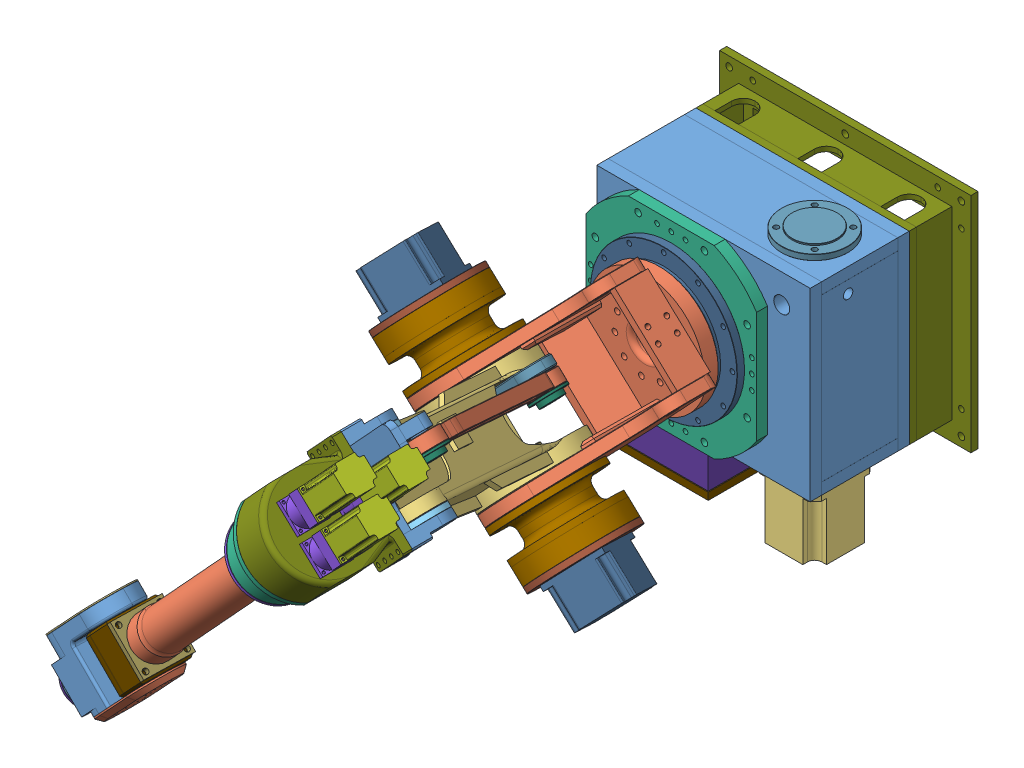
SolidWorks assembly CHX-3装配图, configuration 默认. Lengths in mm.
Overall size (845.77 871.93 1351.14).
99 component instances, 76 part files, 255 mates.
Components (placement in the parent):
- CHX-3底盘旋转涡轮箱-1: CHX-3底盘旋转涡轮箱 [默认] at (-163.7739 242.4792 201.5814) size (450 390 209)
- CHX-3驱动臂座-1: CHX-3驱动臂座 [默认] at (16.2261 47.4792 428.5814) x (-0.730588 0.682819 0) z (0 0 1) size (250 411.05 303.07)
- CHX-3大手臂2-1: CHX-3大手臂2 [默认] at (-120.8336 -194.3627 713.0096) x (0.515271 0.551318 -0.656159) z (-0.730588 0.682819 0) size (210 817.13 178)
- CHX-3小手臂关节轴承-1: CHX-3小手臂关节轴承 [默认] at (145.4781 253.1428 1173.5815) x (0.49992 0.534894 -0.681152) z (-0.730588 0.682819 0) size (72 72 19)
- CHX-3小手臂关节轴承-2: CHX-3小手臂关节轴承 [默认] at (212.6936 190.3221 1173.5815) x (-0.682714 -0.730476 0.017502) z (0.730588 -0.682819 0) size (72 72 19)
- CHX-3小手臂关节轴芯-1: CHX-3小手臂关节轴芯 [默认] at (212.6936 190.3221 1173.5815) x (0.677165 0.724539 0.128414) z (0.730588 -0.682819 0) size (95 95 31)
- CHX-3小手臂关节轴芯-2: CHX-3小手臂关节轴芯 [默认] at (145.4781 253.1428 1173.5815) x (-0.40576 -0.434146 -0.804286) z (-0.730588 0.682819 0) size (95 95 31)
- CHX-3小手臂旋转轴主动齿轮-1: CHX-3小手臂旋转轴主动齿轮 [默认] at (221.5211 267.135 1289.3662) x (0.727771 -0.633712 -0.262218) z (0.677165 0.724539 0.128414) size (28.4 28.27 47)
- CHX-3旋转臂电机-1: CHX-3旋转臂电机 [默认] at (320.3993 416.8662 1282.0229) x (-0.087684 -0.093818 0.991721) z (-0.677165 -0.724539 -0.128414) size (60 60 154.5)
- CHX-3腕部行星减速机-3: CHX-3腕部行星减速机 [默认] at (182.5962 269.4225 1255.8906) x (0.730588 -0.682819 0) z (0.677165 0.724539 0.128414) size (60 60 114)
- CHX-3TVM-611摆线减速机-1: CHX-3TVM-611摆线减速机 [默认] at (-15.3461 -170.831 657.6504) x (0.682819 0.730588 0) z (-0.730588 0.682819 0) size (210 210 176)
- CHX-3TVM-611摆线减速机-2: CHX-3TVM-611摆线减速机 [默认] at (-199.4543 1.2393 657.6504) x (-0.341409 -0.365294 -0.866025) z (0.730588 -0.682819 0) size (210 210 176)
- CHX-3连杆伺服电机-2: CHX-3连杆伺服电机 [默认] at (3.9396 -301.0414 635.6889) x (0.341409 0.365294 0.866025) z (0.730588 -0.682819 0) size (120 120 126.5)
- CHX-3连杆伺服电机-3: CHX-3连杆伺服电机 [默认] at (-259.7091 87.6144 575.6889) x (0.341409 0.365294 0.866025) z (-0.730588 0.682819 0) size (120 120 126.5)
- CHX-3大手臂摆线减速机安装法兰-1: CHX-3大手臂摆线减速机安装法兰 [默认] at (-274.7048 71.5696 657.6504) x (0.341409 0.365294 0.866025) z (0.730588 -0.682819 0) size (204 204 16)
- CHX-3大手臂摆线减速机安装法兰-2: CHX-3大手臂摆线减速机安装法兰 [默认] at (59.9045 -241.1613 657.6504) x (0.341409 0.365294 0.866025) z (-0.730588 0.682819 0) size (204 204 16)
- CHX-3大手臂摆线减速机手臂安装法兰-1: CHX-3大手臂摆线减速机手臂安装法兰 [默认] at (-35.072 -152.3949 657.6504) x (0.669196 0.716013 0.198752) z (-0.730588 0.682819 0) size (135 135 55)
- CHX-3连杆轴承套-1: CHX-3连杆轴承套 [默认] at (-139.546 -54.7518 657.6504) x (0.341409 0.365294 0.866025) z (-0.730588 0.682819 0) size (67 67 55)
- CHX-3连杆轴传动轴-1: CHX-3连杆轴传动轴 [默认] at (-149.0437 -45.8752 657.6504) x (0.678123 0.725564 0.117075) z (0.730588 -0.682819 0) size (235 70 59)
- CHX-3连杆轴承盖-1: CHX-3连杆轴承盖 [默认] at (278.7548 340.0903 1206.6991) x (0.418074 0.447322 0.790644) z (0.730588 -0.682819 0) size (70 70 15)
- CHX-3连杆轴承盖-2: CHX-3连杆轴承盖 [默认] at (-1.3546 40.3847 676.9678) x (0.258501 0.276586 -0.925569) z (0.730588 -0.682819 0) size (70 70 15)
- CHX-3旋转臂电机-2: CHX-3旋转臂电机 [默认] at (286.259 423.5253 1424.4823) x (0.730588 -0.682819 0) z (-0.677165 -0.724539 -0.128414) size (60 60 154.5)
- CHX-3旋转臂电机-3: CHX-3旋转臂电机 [默认] at (343.1408 380.3198 1368.3026) x (-0.087684 -0.093818 0.991721) z (-0.677165 -0.724539 -0.128414) size (60 60 154.5)
- CHX-3腕部行星减速机-4: CHX-3腕部行星减速机 [默认] at (200.0766 227.247 1401.6735) x (0.087684 0.093818 -0.991721) z (0.677165 0.724539 0.128414) size (60 60 114)
- CHX-3腕部行星减速机-5: CHX-3腕部行星减速机 [默认] at (192.2911 235.1125 1398.35) x (-0.730588 0.682819 0) z (0.677165 0.724539 0.128414) size (60 60 114)
- CHX-3腕部电机齿轮箱-1: CHX-3腕部电机齿轮箱 [默认] at (196.3592 240.2128 1348.1206) x (0.730588 -0.682819 0) z (-0.677165 -0.724539 -0.128414) size (210 204.85 98.31)
- CHX-3手腕直齿1-1: CHX-3手腕直齿1 [默认] at (163.8553 205.4349 1341.9567) x (0.440791 -0.259684 -0.859225) z (-0.677165 -0.724539 -0.128414) size (67.8 67.8 20)
- CHX-3手腕直齿3-1: CHX-3手腕直齿3 [默认] at (179.4301 222.0993 1344.9102) x (0.474267 -0.296326 -0.829013) z (-0.677165 -0.724539 -0.128414) size (43.65 43.65 20)
- CHX-3手腕直齿4-1: CHX-3手腕直齿4 [默认] at (192.1209 174.7991 1365.758) x (-0.034964 0.206002 -0.977927) z (-0.677165 -0.724539 -0.128414) size (35.54 35.54 20)
- CHX-3手腕直齿4-2: CHX-3手腕直齿4 [默认] at (153.8046 194.6811 1276.5248) x (0.713515 -0.603899 -0.355249) z (-0.677165 -0.724539 -0.128414) size (35.54 35.54 20)
- CHX-3手腕直齿4-3: CHX-3手腕直齿4 [默认] at (156.0749 240.2981 1365.388) x (-0.708628 0.59511 0.379066) z (-0.677165 -0.724539 -0.128414) size (35.54 35.54 20)
- CHX-3腕部中心轴1-2: CHX-3腕部中心轴1 [默认] at (159.7923 201.0877 1341.1862) x (-0.103765 -0.078746 0.99148) z (-0.677165 -0.724539 -0.128414) size (98 98 563)
- CHX-3腕部中心轴2-1: CHX-3腕部中心轴2 [默认] at (191.6191 235.141 1347.2217) x (0.72823 -0.634867 -0.258119) z (-0.677165 -0.724539 -0.128414) size (20 20 703)
- CHX-3腕部中心轴3-1: CHX-3腕部中心轴3 [默认] at (170.6269 212.6803 1343.2408) x (-0.440791 0.259684 0.859225) z (-0.677165 -0.724539 -0.128414) size (50 50 657.3)
- CHX-3轴承1-1: CHX-3轴承1 [默认] at (129.3199 168.4834 1335.4076) x (0.59922 -0.644269 0.475239) z (-0.677165 -0.724539 -0.128414) size (125 125 18)
- CHX-3轴承1-2: CHX-3轴承1 [默认] at (83.2726 119.2148 1326.6754) x (0.714057 -0.604903 -0.352441) z (-0.677165 -0.724539 -0.128414) size (125 125 18)
- CHX-3小手臂旋转法兰-3: CHX-3小手臂旋转法兰 [默认] at (132.0285 171.3816 1335.9212) x (0.087684 0.093818 -0.991721) z (-0.677165 -0.724539 -0.128414) size (200 180 97)
- CHX-3手腕直齿2-1: CHX-3手腕直齿2 [默认] at (148.2805 188.7705 1339.0032) x (0.441739 -0.539852 0.716538) z (0.677165 0.724539 0.128414) size (97.98 97.94 20)
- CHX-3小手臂旋转轴承法兰-1: CHX-3小手臂旋转轴承法兰 [默认] at (69.7293 104.724 1324.1071) x (0.578605 -0.416486 -0.701252) z (-0.677165 -0.724539 -0.128414) size (155 155 33)
- CHX-3小手臂旋转后法兰-1: CHX-3小手臂旋转后法兰 [默认] at (134.7372 174.2798 1336.4349) x (0.441739 -0.539852 0.716538) z (0.677165 0.724539 0.128414) size (95 95 32)
- CHX-3手腕电机齿轮连接轴-1: CHX-3手腕电机齿轮连接轴 [默认] at (221.239 205.9543 1371.2798) x (0.022963 -0.195239 0.980487) z (-0.677165 -0.724539 -0.128414) size (25 25 53)
- CHX-3手腕电机齿轮连接轴2-1: CHX-3手腕电机齿轮连接轴2 [默认] at (198.4975 242.5007 1285.0001) x (-0.590396 0.639148 -0.492872) z (-0.677165 -0.724539 -0.128414) size (29 29 76)
- CHK-3前爪固定座-2: CHK-3前爪固定座 [默认] at (-245.1525 -232.1867 1264.3944) x (-0.728478 0.68472 -0.021858) z (-0.677165 -0.724539 -0.128414) size (100 100 15.5)
- CHX-3手腕大齿2-1: CHX-3手腕大齿2 [默认] at (-293.2061 -283.602 1255.2818) x (0.440791 -0.259684 -0.859225) z (-0.677165 -0.724539 -0.128414) size (82.68 82.68 53.06)
- CHX-3手腕61908轴承-2: CHX-3手腕61908轴承 [默认] at (-237.0265 -223.4922 1265.9354) x (0.683643 -0.554933 -0.474006) z (-0.677165 -0.724539 -0.128414) size (68 68 12)
- CHX-3手腕61908轴承-3: CHX-3手腕61908轴承 [默认] at (125.2569 164.1362 1334.6371) x (0.658688 -0.519082 -0.544688) z (-0.677165 -0.724539 -0.128414) size (68 68 12)
- CHX-3手腕61908轴承-4: CHX-3手腕61908轴承 [默认] at (-228.9006 -214.7978 1267.4764) x (0.668303 -0.532552 -0.519384) z (-0.677165 -0.724539 -0.128414) size (68 68 12)
- CHX-3手腕61908轴承-5: CHX-3手腕61908轴承 [默认] at (133.3829 172.8307 1336.1781) x (-0.154974 0.311031 -0.937679) z (-0.677165 -0.724539 -0.128414) size (68 68 12)
- CHX-3手腕6002轴承-1: CHX-3手腕6002轴承 [默认] at (164.5325 206.1595 1342.0851) x (0.732546 -0.680269 -0.024713) z (-0.677165 -0.724539 -0.128414) size (32 32 9)
- CHX-3手腕6002轴承-2: CHX-3手腕6002轴承 [默认] at (170.6269 212.6803 1343.2408) x (0.712808 -0.689224 0.129899) z (-0.677165 -0.724539 -0.128414) size (32 32 9)
- CHX-3手腕61902轴承-1: CHX-3手腕61902轴承 [默认] at (-264.9935 -253.4157 1260.6319) x (0.600589 -0.443395 -0.665352) z (-0.677165 -0.724539 -0.128414) size (28 28 7)
- CHX-3手腕61902轴承-2: CHX-3手腕61902轴承 [默认] at (-269.7336 -258.4875 1259.733) x (-0.283367 0.41783 -0.863204) z (-0.677165 -0.724539 -0.128414) size (28 28 7)
- CHX-3手腕小齿-1: CHX-3手腕小齿 [默认] at (-293.2313 -283.629 1255.277) x (-0.601822 0.645756 -0.469905) z (-0.677165 -0.724539 -0.128414) size (42.49 42.49 27.7)
- CHK-3前爪法兰-1: CHK-3前爪法兰 [默认] at (-214.4458 -289.7986 1318.5051) x (-0.677165 -0.724539 -0.128414) z (-0.728478 0.68472 -0.021858) size (112 110 108)
- CHX-3手腕前端旋转法兰-1: CHX-3手腕前端旋转法兰 [默认] at (-315.9608 -183.9595 1200.5471) x (0.728478 -0.68472 0.021858) z (-0.042031 -0.012825 0.999034) size (141 200 110)
- CHK-3前爪法兰侧盖-1: CHK-3前爪法兰侧盖 [默认] at (-305.2348 -395.7723 1253.3323) x (0.683779 0.728693 0.038123) z (-0.728478 0.68472 -0.021858) size (200 110 13)
- CHK-3前爪法兰侧钣金盖-1: CHK-3前爪法兰侧钣金盖 [默认] at (-418.8774 -288.9559 1249.9225) x (0.683779 0.728693 0.038123) z (0.728478 -0.68472 0.021858) size (200 110 2)
- CHX-3小手腕旋转齿轮-2: CHX-3小手腕旋转齿轮 [默认] at (-347.5029 -232.6173 1253.6486) x (0.638355 0.690038 0.341101) z (0.728478 -0.68472 0.021858) size (93.98 93.93 15)
- CHX-3手腕大齿-2-1: CHX-3手腕大齿-2 [默认] at (-293.1855 -283.672 1255.2784) x (0.683779 0.728693 0.038123) z (0.728478 -0.68472 0.021858) size (82.68 82.68 55.06)
- CHX-3手腕轴1-1: CHX-3手腕轴1 [默认] at (-302.4829 -274.933 1254.9994) x (0.638355 0.690038 0.341101) z (-0.728478 0.68472 -0.021858) size (20 20 69.3)
- CHX-3手腕前爪连接轴-1: CHX-3手腕前爪连接轴 [默认] at (-261.9067 -313.072 1256.2169) x (0.683779 0.728693 0.038123) z (0.728478 -0.68472 0.021858) size (62 62 19)
- CHX-3手腕前端锥齿2-1: CHX-3手腕前端锥齿2 [默认] at (-354.7713 -349.2113 1251.846) x (-0.57505 0.570294 -0.586585) z (0.683779 0.728693 0.038123) size (52.79 52.7 37)
- CHX-3小手腕旋转齿轮-2-1: CHX-3小手腕旋转齿轮-2 [默认] at (-409.0429 -298.1997 1250.2175) x (0.655459 0.687358 -0.312909) z (-0.728478 0.68472 -0.021858) size (93.98 93.93 15)
- CHX-3小手腕锥齿轮旋转中心轴-1: CHX-3小手腕锥齿轮旋转中心轴 [默认] at (-414.5065 -293.0643 1250.0536) x (0.655459 0.687358 -0.312909) z (0.728478 -0.68472 0.021858) size (39 39 145)
- CHX-3手腕6007轴承-1: CHX-3手腕6007轴承 [默认] at (-395.5661 -310.867 1250.6219) x (-0.600116 -0.653205 -0.461719) z (-0.728478 0.68472 -0.021858) size (62 62 9)
- CHX-3手腕6204轴承-1: CHX-3手腕6204轴承 [默认] at (-328.5461 -373.8613 1252.6329) x (0.231702 0.276284 0.932728) z (0.728478 -0.68472 0.021858) size (47 47 14)
- CHX-3手腕16011轴承-1: CHX-3手腕16011轴承 [默认] at (-261.9067 -313.072 1256.2169) x (0.164462 0.205767 0.964682) z (0.728478 -0.68472 0.021858) size (90 90 11)
- CHX-3手腕16011轴承-2: CHX-3手腕16011轴承 [默认] at (-332.5691 -246.6541 1254.0967) x (0.272826 0.319233 0.907555) z (0.728478 -0.68472 0.021858) size (90 90 11)
- CHX-3小手腕前端法兰-1: CHX-3小手腕前端法兰 [默认] at (-399.2169 -396.5764 1249.368) x (0.042031 0.012825 -0.999034) z (0.683779 0.728693 0.038123) size (90 90 33)
- CHX-3腕部前端中心轴-1: CHX-3腕部前端中心轴 [默认] at (-366.3956 -361.5991 1251.1979) x (0.57505 -0.570294 0.586585) z (-0.683779 -0.728693 -0.038123) size (60 60 71)
- CHX-3手腕小齿-2: CHX-3手腕小齿 [默认] at (-293.2313 -283.629 1255.277) x (0.638355 0.690038 0.341101) z (0.728478 -0.68472 0.021858) size (42.49 42.49 27.7)
- CHX-3小手臂骨架油封-1: CHX-3小手臂骨架油封 [默认] at (56.8632 90.9578 1321.6672) x (-0.503239 0.583332 -0.637554) z (-0.677165 -0.724539 -0.128414) size (105 105 12)
- CHX-3手腕前端轴承顶套-1: CHX-3手腕前端轴承顶套 [默认] at (-408.7899 -406.7781 1248.8343) x (-0.728478 0.68472 -0.021858) z (0.683779 0.728693 0.038123) size (90 90 16)
- CHX-3手腕前端锥齿1-1: CHX-3手腕前端锥齿1 [默认] at (-354.7713 -349.2113 1251.846) x (-0.655459 -0.687358 0.312909) z (0.728478 -0.68472 0.021858) size (52.79 52.7 37)
- CHX-3腕部中心轴骨架油封-2: CHX-3腕部中心轴骨架油封 [默认] at (-401.9521 -399.4912 1249.2155) x (0.553474 -0.551989 0.623678) z (-0.683779 -0.728693 -0.038123) size (55 55 10)
- CHX-3手腕61907轴承-1: CHX-3手腕61907轴承 [默认] at (-386.9089 -383.4599 1250.0542) x (0.266768 -0.298271 0.916444) z (0.683779 0.728693 0.038123) size (55 55 10)
- CHX-3手腕61907轴承-2: CHX-3手腕61907轴承 [默认] at (-397.8494 -395.119 1249.4442) x (0.266768 -0.298271 0.916444) z (0.683779 0.728693 0.038123) size (55 55 10)
- CHX-3底盘旋转电机SGMGH-13A-B键8X7-1: CHX-3底盘旋转电机SGMGH-13A-B键8X7 [默认] at (256.2261 -170.5208 371.0814) x (0 0 -1) z (0 -1 0) size (130 130 197)
- CHX-3底盘旋转涡轮-1: CHX-3底盘旋转涡轮 [默认] at (16.2261 47.4792 306.0814) x (-0.730588 0.682819 0) z (0 0 -1) size (320.22 320.22 100)
- CHX-3底盘旋转涡杆-1: CHX-3底盘旋转涡杆 [默认] at (191.2261 45.9792 306.0814) x (0.906678 0 -0.421823) z (0 -1 0) size (64 64 391.5)
- CHX-3底盘法兰盖-1: CHX-3底盘法兰盖 [默认] at (36.2261 42.4792 410.5814) size (360 390 23)
- CHX-3底盘旋转涡轮轴-1: CHX-3底盘旋转涡轮轴 [默认] at (16.2261 47.4792 368.0814) x (-0.730588 0.682819 0) z (0 0 -1) size (175 175 332)
- CHX-3底盘旋转涡轮轴下法兰-1: CHX-3底盘旋转涡轮轴下法兰 [默认] at (16.2261 47.4792 227.5814) x (-0.809017 -0.587785 0) z (0 0 -1) size (205 205 79)
- CHX-3底盘旋转51315轴承-2: CHX-3底盘旋转51315轴承 [默认] at (16.2261 47.4792 239.0814) x (0.990498 0.137527 0) z (0 0 1) size (135 135 44)
- CHX-3底盘旋转涡轮轴上法兰盖-1: CHX-3底盘旋转涡轮轴上法兰盖 [默认] at (16.2261 47.4792 449.5814) x (0 -1 0) z (0 0 -1) size (310 310 66)
- CHX-3底盘旋转涡轮轴上法兰16032轴承-2: CHX-3底盘旋转涡轮轴上法兰16032轴承 [默认] at (16.2261 47.4792 396.5814) size (240 240 38)
- CHX-3底盘旋转涡轮轴下法兰6215轴承-1: CHX-3底盘旋转涡轮轴下法兰6215轴承 [默认] at (16.2261 47.4792 153.5814) x (0.976634 0.214912 0) z (0 0 1) size (115 115 20)
- CHX-3底盘旋转涡轮轴下法兰6215轴承-2: CHX-3底盘旋转涡轮轴下法兰6215轴承 [默认] at (16.2261 47.4792 173.5814) size (115 115 20)
- CHX-3底盘旋转涡轮轴上法兰油封-1: CHX-3底盘旋转涡轮轴上法兰油封 [默认] at (16.2261 47.4792 441.5814) size (190 190 14)
- CHX-3底盘旋转涡杆轴承法兰-1: CHX-3底盘旋转涡杆轴承法兰 [默认] at (191.2261 242.4792 306.0814) x (0.707107 0 0.707107) z (0 1 0) size (140 140 44)
- CHX-3底盘旋转涡杆电机法兰-1: CHX-3底盘旋转涡杆电机法兰 [默认] at (191.2261 -147.5208 306.0814) x (0 0 -1) z (0 -1 0) size (130 130 52)
- CHX-3箱体底座-1: CHX-3箱体底座 [默认] at (286.2261 242.4792 186.5814) x (0 -1 0) z (0 0 1) size (470 530 105)
- CHX-3小电箱-1: CHX-3小电箱 [默认] at (-128.7739 -147.5208 410.5814) x (1 0 0) z (0 -1 0) size (200 209 100)
- CHX-3小电箱盖-1: CHX-3小电箱盖 [默认] at (74.2261 -249.5208 413.5814) x (-1 0 0) z (0 1 0) size (206 215 15)
- CHX-3小手臂座-2: CHX-3小手臂座 [Default] at (240.7145 400.439 1261.4789) x (-0.730588 0.682819 0) z (0.087684 0.093818 -0.991721) size (210 230 112.5)
- CHX-3连杆-2: CHX-3连杆 [默认] at (259.0289 358.5264 1206.6991) x (-0.418074 -0.447322 -0.790644) z (0.730588 -0.682819 0) size (740 72.5 27)
- CHX-3小手臂旋转法兰轴承隔套-1: CHX-3小手臂旋转法兰轴承隔套 [默认] at (117.1309 155.4417 1333.0961) x (-0.663165 0.676547 -0.320151) z (-0.677165 -0.724539 -0.128414) size (100 100 50)
- CHX-3腕部中心轴前端锁帽-1: CHX-3腕部中心轴前端锁帽 [默认] at (-250.5698 -237.983 1263.3671) x (0.735823 -0.667557 -0.113719) z (0.677165 0.724539 0.128414) size (56.68 56.68 8)
- CHX-3腕部中心轴前端锁帽-2: CHX-3腕部中心轴前端锁帽 [默认] at (-255.9872 -243.7793 1262.3398) x (-0.327641 0.453154 -0.829037) z (0.677165 0.724539 0.128414) size (56.68 56.68 8)
Mates (geometry in assembly coordinates):
- 同心66: concentric anti-aligned: cylinder of CHX-3大手臂2-1 through (212.6936 190.3221 1173.5815) axis (0.730588 -0.682819 0) radius 36; cylinder of CHX-3小手臂关节轴承-2 through (226.5748 177.3486 1173.5815) axis (-0.730588 0.682819 0) radius 36
- 重合49: coincident aligned: plane of CHX-3大手臂2-1 through (226.5748 177.3486 1173.5815) normal (0.730588 -0.682819 0); plane of CHX-3小手臂关节轴承-2 through (226.5748 177.3486 1173.5815) normal (0.730588 -0.682819 0)
- 同心67: concentric anti-aligned: cylinder of CHX-3大手臂2-1 through (145.4781 253.1428 1173.5815) axis (-0.730588 0.682819 0) radius 36; cylinder of CHX-3小手臂关节轴承-1 through (131.5969 266.1164 1173.5815) axis (0.730588 -0.682819 0) radius 15
- 重合50: coincident aligned: plane of CHX-3大手臂2-1 through (131.5969 266.1164 1173.5815) normal (-0.730588 0.682819 0); plane of CHX-3小手臂关节轴承-1
- 同心70: concentric aligned: cylinder of CHX-3小手臂关节轴承-2 through (226.5748 177.3486 1173.5815) axis (-0.730588 0.682819 0) radius 15; cylinder of CHX-3小手臂关节轴芯-1 through (226.5748 177.3486 1173.5815) axis (-0.730588 0.682819 0) radius 15
- 重合56: coincident anti-aligned: plane of CHX-3小手臂关节轴承-2 through (226.5748 177.3486 1173.5815) normal (0.730588 -0.682819 0); plane of CHX-3小手臂关节轴芯-1 through (226.5748 177.3486 1173.5815) normal (-0.730588 0.682819 0)
- 同心71: concentric aligned: cylinder of CHX-3小手臂关节轴承-1 through (131.5969 266.1164 1173.5815) axis (0.730588 -0.682819 0) radius 15; cylinder of CHX-3小手臂关节轴芯-2 through (131.5969 266.1164 1173.5815) axis (0.730588 -0.682819 0) radius 15
- 重合57: coincident anti-aligned: plane of CHX-3小手臂关节轴承-1; plane of CHX-3小手臂关节轴芯-2
- 同心98: concentric anti-aligned: cylinder of CHX-3小手臂旋转轴主动齿轮-1 through (253.3479 301.1883 1295.4017) axis (-0.677165 -0.724539 -0.128414) radius 10; cylinder of CHX-3旋转臂电机-1 through (235.0644 281.6258 1291.9345) axis (0.677165 0.724539 0.128414) radius 7
- 重合79: coincident anti-aligned: plane of CHX-3小手臂旋转轴主动齿轮-1 through (253.3479 301.1883 1295.4017) normal (0.677165 0.724539 0.128414); plane of CHX-3旋转臂电机-1 through (253.3479 301.1883 1295.4017) normal (-0.677165 -0.724539 -0.128414)
- 同心134: concentric aligned: cylinder of CHX-3旋转臂电机-1 through (235.0644 281.6258 1291.9345) axis (0.677165 0.724539 0.128414) radius 7; cylinder of CHX-3腕部行星减速机-3 through (235.0644 281.6258 1291.9345) axis (0.677165 0.724539 0.128414) radius 7
- 重合114: coincident aligned: plane of CHX-3旋转臂电机-1 through (279.9275 285.6919 1266.0353) normal (0.730588 -0.682819 0); plane of CHX-3腕部行星减速机-3 through (279.9275 285.6919 1266.0353) normal (0.730588 -0.682819 0)
- 重合143: coincident anti-aligned: plane of CHX-3旋转臂电机-1 through (279.9275 285.6919 1266.0353) normal (-0.677165 -0.724539 -0.128414); plane of CHX-3腕部行星减速机-3 through (230.8312 321.032 1325.5385) normal (0.677165 0.724539 0.128414)
- 同心179: concentric aligned: cylinder of CHX-3驱动臂座-1 through (-46.7614 -141.4698 657.6504) axis (0.730588 -0.682819 0) radius 70; cylinder of CHX-3TVM-611摆线减速机-1 through (-75.2543 -114.8399 657.6504) axis (0.730588 -0.682819 0) radius 19
- 同心180: concentric anti-aligned: cylinder of CHX-3驱动臂座-1 through (-189.9566 -7.6374 657.6504) axis (0.730588 -0.682819 0) radius 105; cylinder of CHX-3TVM-611摆线减速机-2 through (-139.546 -54.7518 657.6504) axis (-0.730588 0.682819 0) radius 19
- 同心182: concentric anti-aligned: cylinder of CHX-3驱动臂座-1 through (-24.8437 -161.9544 657.6504) axis (-0.730588 0.682819 0) radius 105; cylinder of CHX-3大手臂2-1 through (-64.2955 -125.0822 657.6504) axis (0.730588 -0.682819 0) radius 105
- 距离19: distance = 1 mm anti-aligned: plane of CHX-3驱动臂座-1 through (-41.6473 -146.2495 657.6504) normal (-0.730588 0.682819 0); plane of CHX-3大手臂2-1 through (-42.3778 -145.5667 657.6504) normal (0.730588 -0.682819 0)
- 同心183: concentric aligned: cylinder of CHX-3TVM-611摆线减速机-2 through (-225.7554 25.8208 657.6504) axis (-0.730588 0.682819 0) radius 9; cylinder of CHX-3连杆伺服电机-3 through (-245.4813 44.2569 657.6504) axis (-0.730588 0.682819 0) radius 9.5
- 同心184: concentric aligned: cylinder of CHX-3TVM-611摆线减速机-1 through (10.9551 -195.4125 657.6504) axis (0.730588 -0.682819 0) radius 9; cylinder of CHX-3连杆伺服电机-2 through (30.681 -213.8486 657.6504) axis (0.730588 -0.682819 0) radius 9.5
- 重合149: coincident anti-aligned: plane of CHX-3驱动臂座-1 through (-24.8437 -161.9544 657.6504) normal (0.730588 -0.682819 0); plane of CHX-3TVM-611摆线减速机-1 through (-24.8437 -161.9544 657.6504) normal (-0.730588 0.682819 0)
- 同心185: concentric aligned: cylinder of CHX-3驱动臂座-1 through (-229.4505 -32.32 735.5927) axis (0.730588 -0.682819 0) radius 5; cylinder of CHX-3TVM-611摆线减速机-1 through (-100.867 -152.4961 735.5927) axis (0.730588 -0.682819 0) radius 5.5
- 同心186: concentric anti-aligned: cylinder of CHX-3驱动臂座-1 through (-229.4505 -32.32 735.5927) axis (0.730588 -0.682819 0) radius 5; cylinder of CHX-3TVM-611摆线减速机-2 through (-175.387 -82.8486 735.5927) axis (-0.730588 0.682819 0) radius 5.5
- 重合150: coincident anti-aligned: plane of CHX-3驱动臂座-1 through (-189.9566 -7.6374 657.6504) normal (-0.730588 0.682819 0); plane of CHX-3TVM-611摆线减速机-2
- 同心187: concentric aligned: cylinder of CHX-3TVM-611摆线减速机-2 through (-262.2848 59.9617 657.6504) axis (-0.730588 0.682819 0) radius 69; cylinder of CHX-3大手臂摆线减速机安装法兰-1 through (-263.746 61.3273 657.6504) axis (-0.730588 0.682819 0) radius 69
- 同心188: concentric aligned: cylinder of CHX-3TVM-611摆线减速机-2 through (-174.7267 84.8129 702.6504) axis (-0.730588 0.682819 0) radius 5.5; cylinder of CHX-3大手臂摆线减速机安装法兰-1 through (-191.5303 100.5177 702.6504) axis (-0.730588 0.682819 0) radius 5
- 同心190: concentric anti-aligned: cylinder of CHX-3连杆伺服电机-3 through (-290.0832 181.7962 676.4148) axis (0.730588 -0.682819 0) radius 5; cylinder of CHX-3大手臂摆线减速机安装法兰-1 through (-221.0426 117.2698 676.4148) axis (-0.730588 0.682819 0) radius 4
- 重合152: coincident anti-aligned: plane of CHX-3连杆伺服电机-3 through (-330.6697 11.6895 635.6889) normal (0.730588 -0.682819 0); plane of CHX-3大手臂摆线减速机安装法兰-1 through (-274.7048 71.5696 657.6504) normal (-0.730588 0.682819 0)
- 同心191: concentric aligned: cylinder of CHX-3TVM-611摆线减速机-1 through (47.4845 -229.5534 657.6504) axis (0.730588 -0.682819 0) radius 69; cylinder of CHX-3大手臂摆线减速机安装法兰-2 through (22.6445 -206.3376 657.6504) axis (0.730588 -0.682819 0) radius 55
- 同心192: concentric aligned: cylinder of CHX-3TVM-611摆线减速机-1 through (13.1468 -197.4609 747.6504) axis (0.730588 -0.682819 0) radius 5.5; cylinder of CHX-3大手臂摆线减速机安装法兰-2 through (29.9504 -213.1657 747.6504) axis (0.730588 -0.682819 0) radius 5
- 同心193: concentric anti-aligned: cylinder of CHX-3连杆伺服电机-2 through (110.2877 -313.9341 727.68) axis (-0.730588 0.682819 0) radius 5; cylinder of CHX-3大手臂摆线减速机安装法兰-2 through (41.2471 -249.4078 727.68) axis (0.730588 -0.682819 0) radius 4
- 重合154: coincident anti-aligned: circle of CHX-3连杆伺服电机-2; plane of CHX-3大手臂摆线减速机安装法兰-2
- 同心194: concentric aligned: cylinder of CHX-3TVM-611摆线减速机-1 through (-75.2543 -114.8399 657.6504) axis (0.730588 -0.682819 0) radius 19; cylinder of CHX-3大手臂摆线减速机手臂安装法兰-1 through (-42.3778 -145.5667 657.6504) axis (0.730588 -0.682819 0) radius 32.5
- 重合156: coincident aligned: plane of CHX-3TVM-611摆线减速机-1 through (-75.2543 -114.8399 657.6504) normal (-0.730588 0.682819 0); plane of CHX-3大手臂摆线减速机手臂安装法兰-1 through (-75.2543 -114.8399 657.6504) normal (-0.730588 0.682819 0)
- 重合157: coincident anti-aligned: plane of CHX-3TVM-611摆线减速机-1 through (51.1374 -232.9675 657.6504) normal (0.730588 -0.682819 0); plane of CHX-3大手臂摆线减速机安装法兰-2 through (51.1374 -232.9675 657.6504) normal (-0.730588 0.682819 0)
- 重合158: coincident anti-aligned: plane of CHX-3TVM-611摆线减速机-2; plane of CHX-3大手臂摆线减速机安装法兰-1
- 同心197: concentric anti-aligned: cylinder of CHX-3TVM-611摆线减速机-2 through (-139.546 -54.7518 657.6504) axis (-0.730588 0.682819 0) radius 19; cylinder of CHX-3连杆轴承套-1 through (-179.7284 -17.1968 657.6504) axis (0.730588 -0.682819 0) radius 30
- 重合161: coincident anti-aligned: plane of CHX-3TVM-611摆线减速机-2 through (-179.7284 -17.1968 657.6504) normal (0.730588 -0.682819 0); plane of CHX-3连杆轴承套-1 through (-179.7284 -17.1968 657.6504) normal (-0.730588 0.682819 0)
- 重合162: coincident aligned: plane of CHX-3TVM-611摆线减速机-2 through (-166.5471 -10.4159 643.8203) normal (0.341409 0.365294 0.866025); plane of CHX-3连杆轴承套-1 through (-130.0177 -44.5569 643.8203) normal (0.341409 0.365294 0.866025)
- 同心199: concentric anti-aligned: cylinder of CHX-3连杆轴承套-1 through (-179.7284 -17.1968 657.6504) axis (0.730588 -0.682819 0) radius 30; cylinder of CHX-3连杆轴传动轴-1 through (-139.546 -54.7518 657.6504) axis (-0.730588 0.682819 0) radius 30
- 重合163: coincident anti-aligned: plane of CHX-3TVM-611摆线减速机-2; plane of CHX-3连杆轴传动轴-1 through (-139.546 -54.7518 657.6504) normal (-0.730588 0.682819 0)
- 同心250: concentric aligned: cylinder of CHX-3旋转臂电机-2 through (206.1851 293.914 1374.8907) axis (0.677165 0.724539 0.128414) radius 7; cylinder of CHX-3腕部行星减速机-5 through (206.1851 293.914 1374.8907) axis (0.677165 0.724539 0.128414) radius 7
- 平行8: parallel aligned: plane of CHX-3旋转臂电机-2 through (245.7872 292.3511 1408.4947) normal (0.730588 -0.682819 0); plane of CHX-3腕部行星减速机-5 through (199.0628 242.3579 1399.6341) normal (0.730588 -0.682819 0)
- 重合193: coincident anti-aligned: plane of CHX-3旋转臂电机-2; plane of CHX-3腕部行星减速机-5
- 同心251: concentric aligned: cylinder of CHX-3旋转臂电机-3 through (257.8059 245.0794 1378.2142) axis (0.677165 0.724539 0.128414) radius 7; cylinder of CHX-3腕部行星减速机-4 through (200.924 184.2181 1367.4274) axis (0.677165 0.724539 0.128414) radius 7
- 平行9: parallel aligned: plane of CHX-3旋转臂电机-3; plane of CHX-3腕部行星减速机-4 through (253.5727 284.4856 1411.8182) normal (-0.087684 -0.093818 0.991721)
- 重合194: coincident anti-aligned: plane of CHX-3旋转臂电机-3 through (302.669 249.1455 1352.315) normal (-0.677165 -0.724539 -0.128414); plane of CHX-3腕部行星减速机-4
- 同心252: concentric aligned: cylinder of CHX-3腕部行星减速机-5 through (149.3032 233.0527 1364.1039) axis (0.677165 0.724539 0.128414) radius 7; cylinder of CHX-3腕部电机齿轮箱-1 through (162.8465 247.5435 1366.6722) axis (0.677165 0.724539 0.128414) radius 25
- 重合198: coincident anti-aligned: plane of CHX-3腕部行星减速机-5 through (197.5522 240.7415 1338.8468) normal (-0.677165 -0.724539 -0.128414); plane of CHX-3腕部电机齿轮箱-1 through (196.3592 240.2128 1348.1206) normal (0.677165 0.724539 0.128414)
- 同心253: concentric aligned: cylinder of CHX-3腕部行星减速机-4 through (200.924 184.2181 1367.4274) axis (0.677165 0.724539 0.128414) radius 7; cylinder of CHX-3腕部电机齿轮箱-1 through (214.4673 198.7089 1369.9957) axis (0.677165 0.724539 0.128414) radius 25
- 重合199: coincident anti-aligned: plane of CHX-3腕部行星减速机-4; plane of CHX-3腕部电机齿轮箱-1 through (196.3592 240.2128 1348.1206) normal (0.677165 0.724539 0.128414)
- 同心254: concentric aligned: cylinder of CHX-3腕部行星减速机-3 through (199.8518 243.9497 1285.2569) axis (0.677165 0.724539 0.128414) radius 25; cylinder of CHX-3腕部电机齿轮箱-1 through (191.7258 235.2553 1283.716) axis (0.677165 0.724539 0.128414) radius 21
- 重合200: coincident anti-aligned: plane of CHX-3腕部行星减速机-3; plane of CHX-3腕部电机齿轮箱-1 through (196.3592 240.2128 1348.1206) normal (0.677165 0.724539 0.128414)
- 同心258: concentric anti-aligned: cylinder of CHX-3腕部行星减速机-5 through (149.3032 233.0527 1364.1039) axis (0.677165 0.724539 0.128414) radius 7; cylinder of CHX-3手腕直齿4-3 through (217.0197 305.5066 1376.9453) axis (-0.677165 -0.724539 -0.128414) radius 7
- 重合201: coincident aligned: plane of CHX-3腕部行星减速机-5 through (149.3032 233.0527 1364.1039) normal (-0.677165 -0.724539 -0.128414); plane of CHX-3手腕直齿4-3 through (149.3032 233.0527 1364.1039) normal (-0.677165 -0.724539 -0.128414)
- 同心259: concentric anti-aligned: cylinder of CHX-3腕部行星减速机-4 through (200.924 184.2181 1367.4274) axis (0.677165 0.724539 0.128414) radius 7; cylinder of CHX-3手腕直齿4-1 through (253.0657 240.0076 1377.3153) axis (-0.677165 -0.724539 -0.128414) radius 7
- 同心260: concentric anti-aligned: cylinder of CHX-3腕部行星减速机-3 through (178.1825 220.7645 1281.1477) axis (0.677165 0.724539 0.128414) radius 7; cylinder of CHX-3手腕直齿4-2 through (214.7494 259.8896 1288.0821) axis (-0.677165 -0.724539 -0.128414) radius 7
- 距离38: distance = 46 mm aligned: plane of CHX-3腕部行星减速机-3; plane of CHX-3手腕直齿4-2
- 同心263: concentric aligned: cylinder of CHX-3腕部中心轴2-1 through (-292.5541 -282.9044 1255.4054) axis (0.677165 0.724539 0.128414) radius 7.5; cylinder of CHX-3腕部中心轴3-1 through (-276.1667 -265.3706 1258.513) axis (0.677165 0.724539 0.128414) radius 12.5
- 重合212: coincident aligned: plane of CHX-3手腕直齿3-1 through (172.6584 214.854 1343.6261) normal (-0.677165 -0.724539 -0.128414); plane of CHX-3手腕直齿4-3 through (149.3032 233.0527 1364.1039) normal (-0.677165 -0.724539 -0.128414)
- 同心264: concentric anti-aligned: cylinder of CHX-3腕部中心轴1-2 through (129.3199 168.4834 1335.4076) axis (-0.677165 -0.724539 -0.128414) radius 45; cylinder of CHX-3轴承1-1 through (117.1309 155.4417 1333.0961) axis (0.677165 0.724539 0.128414) radius 62.5
- 重合213: coincident anti-aligned: plane of CHX-3腕部中心轴1-2 through (129.3199 168.4834 1335.4076) normal (-0.677165 -0.724539 -0.128414); plane of CHX-3轴承1-1 through (129.3199 168.4834 1335.4076) normal (0.677165 0.724539 0.128414)
- 同心265: concentric anti-aligned: cylinder of CHX-3腕部中心轴1-2 through (129.3199 168.4834 1335.4076) axis (-0.677165 -0.724539 -0.128414) radius 45; cylinder of CHX-3轴承1-2 through (71.0837 106.1731 1324.3639) axis (0.677165 0.724539 0.128414) radius 45
- 同心266: concentric aligned: cylinder of CHX-3轴承1-2 through (71.0837 106.1731 1324.3639) axis (0.677165 0.724539 0.128414) radius 62.5; cylinder of CHX-3小手臂旋转法兰-3 through (69.7293 104.724 1324.1071) axis (0.677165 0.724539 0.128414) radius 77.5
- 重合216: coincident anti-aligned: plane of CHX-3腕部电机齿轮箱-1 through (132.0285 171.3816 1335.9212) normal (-0.677165 -0.724539 -0.128414); plane of CHX-3小手臂旋转法兰-3 through (132.0285 171.3816 1335.9212) normal (0.677165 0.724539 0.128414)
- 重合219: coincident aligned: plane of CHX-3腕部中心轴3-1 through (170.6269 212.6803 1343.2408) normal (0.677165 0.724539 0.128414); plane of CHX-3手腕直齿1-1 through (170.6269 212.6803 1343.2408) normal (0.677165 0.724539 0.128414)
- 同心270: concentric anti-aligned: cylinder of CHX-3腕部电机齿轮箱-1 through (188.2332 231.5184 1346.5796) axis (-0.677165 -0.724539 -0.128414) radius 82.5; cylinder of CHX-3小手臂旋转法兰-3 through (52.8002 86.6105 1320.8967) axis (0.677165 0.724539 0.128414) radius 62.5
- 重合220: coincident anti-aligned: plane of CHX-3轴承1-2 through (71.0837 106.1731 1324.3639) normal (-0.677165 -0.724539 -0.128414); plane of CHX-3小手臂旋转轴承法兰-1 through (71.0837 106.1731 1324.3639) normal (0.677165 0.724539 0.128414)
- 同心271: concentric anti-aligned: cylinder of CHX-3手腕直齿3-1 through (240.375 287.3079 1356.4675) axis (-0.677165 -0.724539 -0.128414) radius 7.5; cylinder of CHX-3腕部中心轴2-1 through (-292.5541 -282.9044 1255.4054) axis (0.677165 0.724539 0.128414) radius 7.5
- 同心272: concentric aligned: cylinder of CHX-3腕部中心轴2-1 through (-292.5541 -282.9044 1255.4054) axis (0.677165 0.724539 0.128414) radius 7.5; cylinder of CHX-3腕部中心轴3-1 through (158.438 199.6386 1340.9294) axis (0.677165 0.724539 0.128414) radius 16
- 重合221: coincident anti-aligned: plane of CHX-3小手臂旋转法兰-3 through (69.7293 104.724 1324.1071) normal (-0.677165 -0.724539 -0.128414); plane of CHX-3小手臂旋转轴承法兰-1 through (69.7293 104.724 1324.1071) normal (0.677165 0.724539 0.128414)
- 同心275: concentric aligned: cylinder of CHX-3腕部中心轴1-2 through (60.9262 95.305 1322.4377) axis (-0.677165 -0.724539 -0.128414) radius 40; cylinder of CHX-3小手臂旋转轴承法兰-1 through (73.1151 108.3467 1324.7492) axis (-0.677165 -0.724539 -0.128414) radius 45
- 同心276: concentric aligned: cylinder of CHX-3腕部中心轴1-2 through (159.7923 201.0877 1341.1862) axis (-0.677165 -0.724539 -0.128414) radius 30; cylinder of CHX-3腕部中心轴3-1 through (133.3829 172.8307 1336.1781) axis (-0.677165 -0.724539 -0.128414) radius 20
- 同心277: concentric anti-aligned: cylinder of CHX-3腕部中心轴1-2 through (-246.5068 -233.6358 1264.1376) axis (0.677165 0.724539 0.128414) radius 34; cylinder of CHX-3小手臂旋转后法兰-1 through (141.5088 181.5252 1337.719) axis (-0.677165 -0.724539 -0.128414) radius 47.5
- 重合222: coincident anti-aligned: plane of CHX-3腕部中心轴1-2 through (134.7372 174.2798 1336.4349) normal (0.677165 0.724539 0.128414); plane of CHX-3小手臂旋转后法兰-1 through (134.7372 174.2798 1336.4349) normal (-0.677165 -0.724539 -0.128414)
- 重合225: coincident aligned: plane of CHX-3小手臂旋转后法兰-1 through (133.3829 172.8307 1336.1781) normal (-0.677165 -0.724539 -0.128414); plane of CHX-3腕部中心轴3-1 through (133.3829 172.8307 1336.1781) normal (-0.677165 -0.724539 -0.128414)
- 同心282: concentric aligned: cylinder of CHX-3腕部行星减速机-4 through (200.924 184.2181 1367.4274) axis (0.677165 0.724539 0.128414) radius 7; cylinder of CHX-3手腕电机齿轮连接轴-1 through (198.8925 182.0445 1367.0421) axis (0.677165 0.724539 0.128414) radius 12.5
- 重合227: coincident anti-aligned: plane of CHX-3腕部行星减速机-4 through (221.239 205.9543 1371.2798) normal (-0.677165 -0.724539 -0.128414); plane of CHX-3手腕电机齿轮连接轴-1 through (221.239 205.9543 1371.2798) normal (0.677165 0.724539 0.128414)
- 重合228: coincident aligned: plane of CHX-3手腕直齿4-1; plane of CHX-3手腕电机齿轮连接轴-1 through (185.3492 167.5537 1364.4739) normal (-0.677165 -0.724539 -0.128414)
- 同心283: concentric aligned: cylinder of CHX-3腕部行星减速机-3 through (178.1825 220.7645 1281.1477) axis (0.677165 0.724539 0.128414) radius 7; cylinder of CHX-3手腕电机齿轮连接轴2-1 through (160.5762 201.9265 1277.8089) axis (0.677165 0.724539 0.128414) radius 12.5
- 重合229: coincident anti-aligned: plane of CHX-3腕部行星减速机-3; plane of CHX-3手腕电机齿轮连接轴2-1 through (198.4975 242.5007 1285.0001) normal (0.677165 0.724539 0.128414)
- 平行13: parallel aligned: plane of CHX-3腕部电机齿轮箱-1 through (267.7221 184.7616 1284.6703) normal (0.730588 -0.682819 0); plane of CHX-3小手臂旋转法兰-3 through (205.9126 118.628 1454.2126) normal (0.730588 -0.682819 0)
- 同心309: concentric anti-aligned: cylinder of CHX-3腕部中心轴1-2 through (-228.9006 -214.7978 1267.4764) axis (-0.677165 -0.724539 -0.128414) radius 34; cylinder of CHX-3手腕61908轴承-4 through (-237.0265 -223.4922 1265.9354) axis (0.677165 0.724539 0.128414) radius 22.5
- 同心310: concentric anti-aligned: cylinder of CHX-3腕部中心轴1-2 through (-228.9006 -214.7978 1267.4764) axis (-0.677165 -0.724539 -0.128414) radius 34; cylinder of CHX-3手腕61908轴承-2 through (-245.1525 -232.1867 1264.3944) axis (0.677165 0.724539 0.128414) radius 22.5
- 重合238: coincident anti-aligned: plane of CHX-3腕部中心轴1-2 through (-228.9006 -214.7978 1267.4764) normal (-0.677165 -0.724539 -0.128414); plane of CHX-3手腕61908轴承-4 through (-228.9006 -214.7978 1267.4764) normal (0.677165 0.724539 0.128414)
- 重合239: coincident anti-aligned: plane of CHX-3手腕61908轴承-2; plane of CHX-3手腕61908轴承-4 through (-237.0265 -223.4922 1265.9354) normal (-0.677165 -0.724539 -0.128414)
- 同心311: concentric aligned: cylinder of CHX-3腕部中心轴1-2 through (-246.5068 -233.6358 1264.1376) axis (0.677165 0.724539 0.128414) radius 34; cylinder of CHX-3手腕61908轴承-5 through (125.2569 164.1362 1334.6371) axis (0.677165 0.724539 0.128414) radius 34
- 同心312: concentric aligned: cylinder of CHX-3腕部中心轴1-2 through (-246.5068 -233.6358 1264.1376) axis (0.677165 0.724539 0.128414) radius 34; cylinder of CHX-3手腕61908轴承-3 through (117.1309 155.4417 1333.0961) axis (0.677165 0.724539 0.128414) radius 34
- 重合240: coincident anti-aligned: plane of CHX-3腕部中心轴1-2 through (117.1309 155.4417 1333.0961) normal (0.677165 0.724539 0.128414); plane of CHX-3手腕61908轴承-3
- 重合241: coincident anti-aligned: plane of CHX-3手腕61908轴承-3; plane of CHX-3手腕61908轴承-5
- 同心314: concentric aligned: cylinder of CHX-3腕部中心轴3-1 through (158.438 199.6386 1340.9294) axis (0.677165 0.724539 0.128414) radius 16; cylinder of CHX-3手腕6002轴承-2 through (164.5325 206.1595 1342.0851) axis (0.677165 0.724539 0.128414) radius 16
- 同心315: concentric aligned: cylinder of CHX-3腕部中心轴3-1 through (158.438 199.6386 1340.9294) axis (0.677165 0.724539 0.128414) radius 16; cylinder of CHX-3手腕6002轴承-1 through (158.438 199.6386 1340.9294) axis (0.677165 0.724539 0.128414) radius 16
- 重合242: coincident anti-aligned: plane of CHX-3腕部中心轴3-1 through (158.438 199.6386 1340.9294) normal (0.677165 0.724539 0.128414); plane of CHX-3手腕6002轴承-1 through (158.438 199.6386 1340.9294) normal (-0.677165 -0.724539 -0.128414)
- 重合243: coincident anti-aligned: plane of CHX-3手腕6002轴承-1 through (164.5325 206.1595 1342.0851) normal (0.677165 0.724539 0.128414); plane of CHX-3手腕6002轴承-2
- 重合246: coincident anti-aligned: plane of CHX-3腕部中心轴3-1 through (-264.9935 -253.4157 1260.6319) normal (-0.677165 -0.724539 -0.128414); plane of CHX-3手腕61902轴承-1 through (-264.9935 -253.4157 1260.6319) normal (0.677165 0.724539 0.128414)
- 同心321: concentric aligned: cylinder of CHX-3腕部中心轴2-1 through (-292.5541 -282.9044 1255.4054) axis (0.677165 0.724539 0.128414) radius 7.5; cylinder of CHX-3手腕61902轴承-1 through (-269.7336 -258.4875 1259.733) axis (0.677165 0.724539 0.128414) radius 7.5
